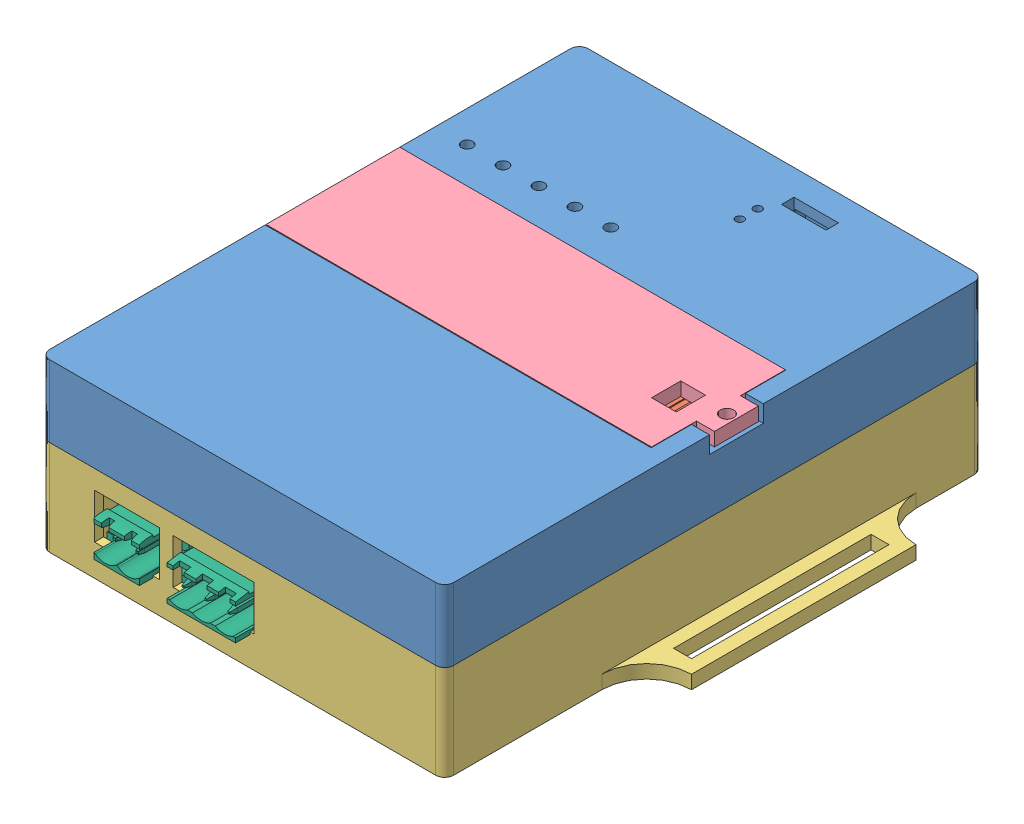
SolidWorks assembly Assem1, configuration Default. Lengths in mm.
Overall size (110 38.9 123.27).
16 component instances, 8 part files, 33 mates.
Components (placement in the parent):
- top-1: top [Default] at (-2.8808 61.6563 149.0822) size (90 16 120)
- TTGO_SIM7000GV1-1: TTGO_SIM7000GV1 [Default] at (91.0661 -44.1203 96.2055) x (0 0 1) z (-1 0 0) size (110.54 27.81 45.55)
- bottom-1: bottom [Default] at (87.1192 39.4563 149.0822) x (0 0 -1) z (1 0 0) size (120 22.2 110)
- top cover-1: top cover [Default] at (-2.8808 76.6563 69.0822) x (1 0 0) z (0 0 -1) size (89.9 11.5 29.8)
- PCB222-1: PCB222 [Default] at (1.1179 68.6563 64.0822) x (1 0 0) z (0 1 0) size (37.95 26.39 7.52)
- PCB111111111-1: PCB111111111 [Default] at (-0.0178 44.4563 145.2862) x (1 0 0) z (0 1 0) size (55.93 79.53 17.5)
- M4 threaded insert (1)-1: M4 threaded insert (1) [Default] at (2.6192 61.9563 34.5822) x (-0.96242 0 0.271566) z (0.271566 0 0.96242) size (5.89 7.6 5.89)
- M4 threaded insert (1)-2: M4 threaded insert (1) [Default] at (2.6192 61.9563 143.5822) x (-0.96242 0 0.271566) z (0.271566 0 0.96242) size (5.89 7.6 5.89)
- M4 threaded insert (1)-3: M4 threaded insert (1) [Default] at (81.6192 61.9563 34.5822) x (-0.96242 0 0.271566) z (0.271566 0 0.96242) size (5.89 7.6 5.89)
- M4 threaded insert (1)-4: M4 threaded insert (1) [Default] at (81.6192 61.9563 143.5822) x (-0.96242 0 0.271566) z (0.271566 0 0.96242) size (5.89 7.6 5.89)
- M2 threaded insert123-1: M2 threaded insert123 [Default] at (3.9192 41.9563 91.6822) x (0.986827 0 -0.161782) z (0 1 0) size (4.1 4.1 5.11)
- M2 threaded insert123-2: M2 threaded insert123 [Default] at (52.1192 41.9563 132.3322) x (0.986827 0 -0.161782) z (0 1 0) size (4.1 4.1 5.11)
- M2 threaded insert123-3: M2 threaded insert123 [Default] at (3.9192 41.9563 132.3322) x (0.986827 0 -0.161782) z (0 1 0) size (4.1 4.1 5.11)
- M2 threaded insert123-4: M2 threaded insert123 [Default] at (52.1192 41.9563 91.6822) x (0.986827 0 -0.161782) z (0 1 0) size (4.1 4.1 5.11)
- M2 threaded insert123-5: M2 threaded insert123 [Default] at (48.3092 64.4563 142.2535) x (-0.984078 0 -0.177737) z (0 -1 0) size (4.1 4.1 5.11)
- M2 threaded insert123-6: M2 threaded insert123 [Default] at (76.0192 64.4563 36.6735) x (-0.533663 0 -0.845697) z (0 -1 0) size (4.1 4.1 5.11)
Mates (geometry in assembly coordinates):
- Coincident8: coincident aligned: plane of top-1 through (87.1192 76.6563 149.0822) normal (1 0 0); plane of bottom-1 through (87.1192 61.6563 149.0822) normal (1 0 0)
- Coincident9: coincident aligned: plane of top-1 through (-2.8808 76.6563 149.0822) normal (0 0 1); plane of bottom-1 through (87.1192 61.6563 149.0822) normal (0 0 1)
- Coincident12: coincident aligned: plane of top-1 through (-2.8808 76.6563 149.0822) normal (0 1 0); plane of top cover-1 through (-2.8808 76.6563 69.0822) normal (0 1 0)
- Coincident15: coincident anti-aligned: plane of top-1 through (-2.8808 64.6563 69.0822) normal (0 0 1); plane of top cover-1 through (-2.8808 73.6563 69.0822) normal (0 0 -1)
- Coincident26: coincident aligned: plane of top-1 through (-2.8808 76.6563 149.0822) normal (-1 0 0); plane of top cover-1 through (-2.8808 73.6563 98.8822) normal (-1 0 0)
- Coincident27: coincident anti-aligned: plane of top-1 through (45.7192 66.6563 66.6822) normal (1 0 0); plane of TTGO_SIM7000GV1-1 through (45.7192 63.1339 36.1835) normal (-1 0 0)
- Coincident28: coincident anti-aligned: plane of bottom-1 through (3.9192 44.4563 132.3322) normal (0 1 0); plane of PCB111111111-1 through (27.7892 44.4563 108.2815) normal (0 -1 0)
- Concentric1: concentric anti-aligned: cylinder of bottom-1 through (3.9192 44.4563 132.3322) axis (0 -1 0) radius 3; cylinder of PCB111111111-1 through (3.9192 44.4563 132.3322) axis (0 1 0) radius 1.5
- Parallel1: parallel anti-aligned: cylinder of bottom-1 through (3.9192 44.4563 91.6822) axis (0 -1 0) radius 3; cylinder of PCB111111111-1 through (3.9192 44.4563 91.8191) axis (0 1 0) radius 1.5
- Concentric3: concentric anti-aligned: cylinder of top-1 through (4.1192 73.6563 61.0822) axis (0 1 0) radius 1.25; cylinder of PCB222-1 through (4.1192 74.2563 61.0822) axis (0 -1 0) radius 1.5
- Parallel2: parallel anti-aligned: plane of top-1 through (-0.4808 76.6563 149.0822) normal (1 0 0); plane of PCB222-1 through (1.1306 68.6563 64.0695) normal (-1 0 0)
- Distance1: distance = 3.2 mm anti-aligned: plane of top-1 through (-2.8808 74.4563 149.0822) normal (0 -1 0); plane of PCB222-1 through (4.1192 71.2563 61.0822) normal (0 1 0)
- Coincident31: coincident anti-aligned: plane of top-1 through (-2.8808 60.6563 149.0822) normal (0 -1 0); plane of bottom-1 through (87.1192 60.6563 149.0822) normal (0 1 0)
- Coincident34: coincident anti-aligned: plane of top-1 through (-2.8808 61.9563 149.0822) normal (0 -1 0); circle of M4 threaded insert (1)-1
- Concentric4: concentric aligned: cylinder of top-1 through (2.6192 67.9563 34.5822) axis (0 -1 0) radius 2.5; cylinder of M4 threaded insert (1)-1 through (2.6192 62.4563 34.5822) axis (0 -1 0) radius 2
- Concentric5: concentric aligned: cylinder of top-1 through (81.6192 67.9563 34.5822) axis (0 -1 0) radius 2.5; cylinder of M4 threaded insert (1)-3 through (81.6192 62.4563 34.5822) axis (0 -1 0) radius 2
- Coincident36: coincident anti-aligned: plane of top-1 through (-2.8808 61.9563 149.0822) normal (0 -1 0); circle of M4 threaded insert (1)-3
- Coincident37: coincident anti-aligned: plane of top-1 through (-2.8808 61.9563 149.0822) normal (0 -1 0); circle of M4 threaded insert (1)-4
- Concentric6: concentric aligned: cylinder of top-1 through (81.6192 67.9563 143.5822) axis (0 -1 0) radius 2.5; cylinder of M4 threaded insert (1)-4 through (81.6192 62.4563 143.5822) axis (0 -1 0) radius 2
- Coincident38: coincident anti-aligned: plane of top-1 through (-2.8808 61.9563 149.0822) normal (0 -1 0); circle of M4 threaded insert (1)-2
- Concentric8: concentric anti-aligned: cylinder of top-1 through (2.6192 67.9563 143.5822) axis (0 -1 0) radius 2.5; cone of M4 threaded insert (1)-2 through (2.6192 62.6795 143.5822) axis (0 1 0)
- Coincident39: coincident aligned: plane of bottom-1 through (3.9192 44.4563 91.6822) normal (0 1 0); plane of M2 threaded insert123-1 through (3.9192 44.4563 91.6822) normal (0 1 0)
- Concentric9: concentric anti-aligned: cylinder of bottom-1 through (3.9192 42.4563 91.6822) axis (0 1 0) radius 1.55; circle of M2 threaded insert123-1
- Concentric10: concentric anti-aligned: cylinder of bottom-1 through (52.1192 42.4563 91.6822) axis (0 1 0) radius 1.55; circle of M2 threaded insert123-4
- Coincident40: coincident aligned: plane of bottom-1 through (52.1192 44.4563 91.6822) normal (0 1 0); plane of M2 threaded insert123-4 through (52.1192 44.4563 91.6822) normal (0 1 0)
- Concentric11: concentric anti-aligned: cylinder of bottom-1 through (3.9192 42.4563 132.3322) axis (0 1 0) radius 1.55; circle of M2 threaded insert123-3
- Coincident41: coincident aligned: plane of bottom-1 through (3.9192 44.4563 132.3322) normal (0 1 0); plane of M2 threaded insert123-3 through (3.9192 44.4563 132.3322) normal (0 1 0)
- Concentric12: concentric anti-aligned: cylinder of bottom-1 through (52.1192 42.4563 132.3322) axis (0 1 0) radius 1.55; circle of M2 threaded insert123-2
- Coincident42: coincident aligned: plane of bottom-1 through (52.1192 44.4563 132.3322) normal (0 1 0); plane of M2 threaded insert123-2 through (52.1192 44.4563 132.3322) normal (0 1 0)
- Concentric13: concentric anti-aligned: cylinder of top-1 through (48.3092 64.9563 142.2535) axis (0 -1 0) radius 1.5; circle of M2 threaded insert123-5
- Coincident43: coincident aligned: plane of top-1 through (-2.8808 61.9563 149.0822) normal (0 -1 0); plane of M2 threaded insert123-5 through (48.3092 61.9563 142.2535) normal (0 -1 0)
- Concentric14: concentric anti-aligned: cylinder of top-1 through (76.0192 64.9563 36.6735) axis (0 -1 0) radius 1.5; circle of M2 threaded insert123-6
- Coincident44: coincident aligned: plane of top-1 through (-2.8808 61.9563 149.0822) normal (0 -1 0); plane of M2 threaded insert123-6 through (76.0192 61.9563 36.6735) normal (0 -1 0)
